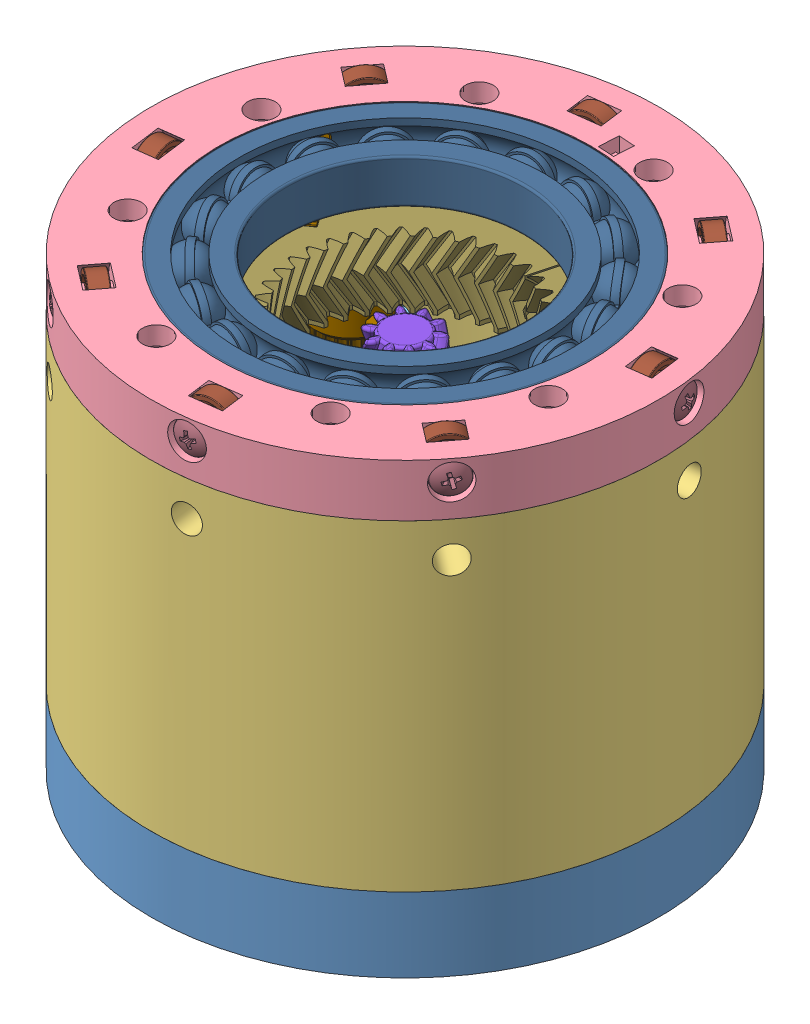
SolidWorks assembly A1 - Final Assembly, configuration Default. Lengths in mm.
Overall size (210.32 133.5 210.32).
45 component instances, 13 part files, 38 mates.
Components (placement in the parent):
- A1D1 - Bottom-1: A1D1 - Bottom [Default] at origin size (150 22 150)
- Turnigy Aerodrive SK3 4250-1: Turnigy Aerodrive SK3 4250 [Default] at (0 73.3 0) x (-0.707107 0 -0.707107) z (-0.707107 0 0.707107) size (52.1 79.08 41.8)
- A1D2 - Middle-1: A1D2 - Middle [Default] at (0 22 0) x (0.991445 0 -0.130526) z (0.130526 0 0.991445) size (150 96 150)
- A1D3 - Top-1: A1D3 - Top [Default] at (0 117 0) x (0.793353 0 0.608761) z (-0.608761 0 0.793353) size (150 15.5 150)
- A1D4 - Encoder bracket-1: A1D4 - Encoder bracket [Default] at (0 30 0) x (0.991445 0 -0.130526) z (0.130526 0 0.991445) size (52.04 50 76.58)
- Encoder600PR-1: Encoder600PR [Default] at (-40.4994 32.32 -24.4547) x (0.84353 0 0.537082) z (-0.537082 0 0.84353) size (38 53 38)
- A1P1_S1 - BLDC Axis Bottom (50T HTD3m)-1: A1P1_S1 - BLDC Axis Bottom (50T HTD3m) [Default] at (-3.3955 88.2939 1.3517) x (0.767493 0 -0.641057) z (0 -1 0) size (46.98 46.92 14.7)
- A1P1_S2 - BLDC Axis Top (Sun in A1R1)-1: A1P1_S2 - BLDC Axis Top (Sun in A1R1) [Default] at (-3.3955 88.2939 1.3517) x (0.767493 0 -0.641057) z (0 -1 0) size (38.1 38.1 28.24)
- A1P2 - Encoder Axis (20T HTD3m)-1: A1P2 - Encoder Axis (20T HTD3m) [Default] at (-40.4994 73.3 -24.4547) x (0.825705 0 -0.564102) z (0 1 0) size (21.34 40.98 60.33)
- radial ball bearing_68_am-3: radial ball bearing_68_am [AFBMA 20.1 - 00-70 - 18,DE,AC,18_68] at (0 126 0) x (0 1 0) z (0 0 1) size (13.2 110 110)
- radial ball bearing_68_iso-1: radial ball bearing_68_iso [ISO 15 RBB - 105 - 8,SI,NC,8_68] at (8.4842 126.5 64.4439) x (0.130526 0 0.991445) z (-0.991445 0 0.130526) size (5 14 14)
- radial ball bearing_68_iso-2: radial ball bearing_68_iso [ISO 15 RBB - 105 - 8,SI,NC,8_68] at (51.568 126.5 39.5695) x (0.793353 0 0.608761) z (-0.608761 0 0.793353) size (5 14 14)
- radial ball bearing_68_iso-3: radial ball bearing_68_iso [ISO 15 RBB - 105 - 8,SI,NC,8_68] at (64.4439 126.5 -8.4842) x (0.991445 0 -0.130526) z (0.130526 0 0.991445) size (5 14 14)
- radial ball bearing_68_iso-4: radial ball bearing_68_iso [ISO 15 RBB - 105 - 8,SI,NC,8_68] at (39.5695 126.5 -51.568) x (0.608761 0 -0.793353) z (0.793353 0 0.608761) size (5 14 14)
- radial ball bearing_68_iso-5: radial ball bearing_68_iso [ISO 15 RBB - 105 - 8,SI,NC,8_68] at (-8.4842 126.5 -64.4439) x (-0.130526 0 -0.991445) z (0.991445 0 -0.130526) size (5 14 14)
- radial ball bearing_68_iso-6: radial ball bearing_68_iso [ISO 15 RBB - 105 - 8,SI,NC,8_68] at (-51.568 126.5 -39.5695) x (-0.793353 0 -0.608761) z (0.608761 0 -0.793353) size (5 14 14)
- radial ball bearing_68_iso-7: radial ball bearing_68_iso [ISO 15 RBB - 105 - 8,SI,NC,8_68] at (-64.4439 126.5 8.4842) x (-0.991445 0 0.130526) z (-0.130526 0 -0.991445) size (5 14 14)
- radial ball bearing_68_iso-8: radial ball bearing_68_iso [ISO 15 RBB - 105 - 8,SI,NC,8_68] at (-39.5695 126.5 51.568) x (-0.608761 0 0.793353) z (-0.793353 0 -0.608761) size (5 14 14)
- A1R1 - Fixed ring (38T)-1: A1R1 - Fixed ring (38T) [Default] at (-96.4762 151.2552 -44.9758) x (0.965926 0 0.258819) z (0 1 0) size (84.14 84.14 19.84)
- pan head cross recess screw_iso-3: pan head cross recess screw_iso [ISO 7045 - M5 x 16 - Z - 16N] at (9.7764 126.5 74.2592) x (-0.130526 0 -0.991445) z (0.264332 -0.963804 -0.0348) size (19.63 9.5 9.5)
- pan head cross recess screw_iso-5: pan head cross recess screw_iso [ISO 7045 - M4 x 16 - Z - 16N] at (6.8787 106.5867 52.2491) x (-0.130526 0 -0.991445) z (-0.096727 -0.995229 0.012734) size (19.02 8 8)
- pan head cross recess screw_iso-6: pan head cross recess screw_iso [ISO 7045 - M4 x 16 - Z - 16N] at (30 128.5 51.9615) x (0 -1 0) z (0.614442 0 0.788962) size (19.02 8 8)
- pan head cross recess screw_iso-7: pan head cross recess screw_iso [ISO 7045 - M4 x 16 - Z - 16N] at (41.8097 106.5867 32.0817) x (-0.793353 0 -0.608761) z (-0.059392 -0.995229 0.077401) size (19.02 8 8)
- pan head cross recess screw_iso-8: pan head cross recess screw_iso [ISO 7045 - M4 x 16 - Z - 16N] at (52.2491 106.5867 -6.8787) x (-0.991445 0 0.130526) z (0.012734 -0.995229 0.096727) size (19.02 8 8)
- pan head cross recess screw_iso-9: pan head cross recess screw_iso [ISO 7045 - M4 x 16 - Z - 16N] at (32.0817 106.5867 -41.8097) x (-0.608761 0 0.793353) z (0.077401 -0.995229 0.059392) size (19.02 8 8)
- pan head cross recess screw_iso-10: pan head cross recess screw_iso [ISO 7045 - M4 x 16 - Z - 16N] at (-6.8787 106.5867 -52.2491) x (0.130526 0 0.991445) z (0.096727 -0.995229 -0.012734) size (19.02 8 8)
- pan head cross recess screw_iso-11: pan head cross recess screw_iso [ISO 7045 - M4 x 16 - Z - 16N] at (-41.8097 106.5867 -32.0817) x (0.793353 0 0.608761) z (0.059392 -0.995229 -0.077401) size (19.02 8 8)
- pan head cross recess screw_iso-12: pan head cross recess screw_iso [ISO 7045 - M4 x 16 - Z - 16N] at (-52.2491 106.5867 6.8787) x (0.991445 0 -0.130526) z (-0.012734 -0.995229 -0.096727) size (19.02 8 8)
- pan head cross recess screw_iso-13: pan head cross recess screw_iso [ISO 7045 - M4 x 16 - Z - 16N] at (-32.0817 106.5867 41.8097) x (0.608761 0 -0.793353) z (-0.077401 -0.995229 -0.059392) size (19.02 8 8)
- pan head cross recess screw_iso-14: pan head cross recess screw_iso [ISO 7045 - M4 x 16 - Z - 16N] at (57.9555 128.5 15.5291) x (0 -1 0) z (0.992357 0 0.123404) size (19.02 8 8)
- pan head cross recess screw_iso-15: pan head cross recess screw_iso [ISO 7045 - M4 x 16 - Z - 16N] at (51.9615 128.5 -30) x (0 -1 0) z (0.788962 0 -0.614442) size (19.02 8 8)
- pan head cross recess screw_iso-16: pan head cross recess screw_iso [ISO 7045 - M4 x 16 - Z - 16N] at (15.5291 128.5 -57.9555) x (0 -1 0) z (0.123404 0 -0.992357) size (19.02 8 8)
- pan head cross recess screw_iso-17: pan head cross recess screw_iso [ISO 7045 - M4 x 16 - Z - 16N] at (-30 128.5 -51.9615) x (0 -1 0) z (-0.614442 0 -0.788962) size (19.02 8 8)
- pan head cross recess screw_iso-18: pan head cross recess screw_iso [ISO 7045 - M4 x 16 - Z - 16N] at (-57.9555 128.5 -15.5291) x (0 -1 0) z (-0.992357 0 -0.123404) size (19.02 8 8)
- pan head cross recess screw_iso-19: pan head cross recess screw_iso [ISO 7045 - M4 x 16 - Z - 16N] at (-51.9615 128.5 30) x (0 -1 0) z (-0.788962 0 0.614442) size (19.02 8 8)
- pan head cross recess screw_iso-20: pan head cross recess screw_iso [ISO 7045 - M4 x 16 - Z - 16N] at (-15.5291 128.5 57.9555) x (0 -1 0) z (-0.123404 0 0.992357) size (19.02 8 8)
- pan head cross recess screw_iso-21: pan head cross recess screw_iso [ISO 7045 - M5 x 16 - Z - 16N] at (59.4222 126.5 45.5962) x (-0.793353 0 -0.608761) z (0.162304 -0.963804 -0.211518) size (19.63 9.5 9.5)
- pan head cross recess screw_iso-22: pan head cross recess screw_iso [ISO 7045 - M5 x 16 - Z - 16N] at (74.2592 126.5 -9.7764) x (-0.991445 0 0.130526) z (-0.0348 -0.963804 -0.264332) size (19.63 9.5 9.5)
- pan head cross recess screw_iso-23: pan head cross recess screw_iso [ISO 7045 - M5 x 16 - Z - 16N] at (45.5962 126.5 -59.4222) x (-0.608761 0 0.793353) z (-0.211518 -0.963804 -0.162304) size (19.63 9.5 9.5)
- pan head cross recess screw_iso-24: pan head cross recess screw_iso [ISO 7045 - M5 x 16 - Z - 16N] at (-9.7764 126.5 -74.2592) x (0.130526 0 0.991445) z (-0.264332 -0.963804 0.0348) size (19.63 9.5 9.5)
- pan head cross recess screw_iso-25: pan head cross recess screw_iso [ISO 7045 - M5 x 16 - Z - 16N] at (-59.4222 126.5 -45.5962) x (0.793353 0 0.608761) z (-0.162304 -0.963804 0.211518) size (19.63 9.5 9.5)
- pan head cross recess screw_iso-26: pan head cross recess screw_iso [ISO 7045 - M5 x 16 - Z - 16N] at (-74.2592 126.5 9.7764) x (0.991445 0 -0.130526) z (0.0348 -0.963804 0.264332) size (19.63 9.5 9.5)
- pan head cross recess screw_iso-27: pan head cross recess screw_iso [ISO 7045 - M5 x 16 - Z - 16N] at (-45.5962 126.5 59.4222) x (0.608761 0 -0.793353) z (0.211518 -0.963804 0.162304) size (19.63 9.5 9.5)
- pan head cross recess screw_iso-29: pan head cross recess screw_iso [ISO 7045 - M5 x 16 - Z - 16N] at (-75.73 69.5 20.0563) x (0.991445 0 -0.130526) z (-0.041237 0.948782 -0.313228) size (19.63 9.5 9.5)
- pan head cross recess screw_iso-30: pan head cross recess screw_iso [ISO 7045 - M5 x 16 - Z - 16N] at (-78.3405 69.5 0.2274) x (0.991445 0 -0.130526) z (0.119155 0.408217 0.905075) size (19.63 9.5 9.5)
Mates (geometry in assembly coordinates):
- Concentric1: concentric anti-aligned: cylinder of A1D1 - Bottom-1 through (-12.5 16 0) axis (0 1 0) radius 1.6; cylinder of Turnigy Aerodrive SK3 4250-1 through (-12.5 24 0) axis (0 -1 0) radius 1.5
- Concentric2: concentric anti-aligned: cylinder of A1D1 - Bottom-1 through (12.5 16 0) axis (0 1 0) radius 1.6; cylinder of Turnigy Aerodrive SK3 4250-1 through (12.5 24 0) axis (0 -1 0) radius 1.5
- Coincident1: coincident anti-aligned: plane of A1D1 - Bottom-1 through (0 22 0) normal (0 1 0); plane of Turnigy Aerodrive SK3 4250-1 through (0 22 0) normal (0 -1 0)
- Concentric3: concentric aligned: cylinder of A1D1 - Bottom-1 through (30 -31.885 51.9615) axis (0 1 0) radius 2.05; cylinder of A1D2 - Middle-1 through (30 21.999 51.9615) axis (0 1 0) radius 2.05
- Concentric4: concentric aligned: cylinder of A1D1 - Bottom-1 through (60 -23.7417 0) axis (0 1 0) radius 2.05; cylinder of A1D2 - Middle-1 through (60 21.999 0) axis (0 1 0) radius 2.05
- Coincident2: coincident anti-aligned: plane of A1D1 - Bottom-1 through (0 22 0) normal (0 1 0); plane of A1D2 - Middle-1 through (-9.7895 22 -74.3584) normal (0 -1 0)
- Concentric5: concentric aligned: cylinder of A1D2 - Middle-1 through (0 22 0) axis (0 -1 0) radius 75; cylinder of A1D3 - Top-1 through (0 132.5 0) axis (0 -1 0) radius 75
- Coincident3: coincident anti-aligned: plane of A1D2 - Middle-1 through (-5.717 117 -43.4253) normal (0 1 0); plane of A1D3 - Top-1 through (0 117 0) normal (0 -1 0)
- Concentric6: concentric aligned: cylinder of A1D2 - Middle-1 through (30 21.999 51.9615) axis (0 1 0) radius 2.05; cylinder of A1D3 - Top-1 through (30 117 51.9615) axis (0 1 0) radius 2.05
- Concentric7: concentric anti-aligned: cylinder of A1D2 - Middle-1 through (-73.0541 69.5 19.704) axis (0.991445 0 -0.130526) radius 2.55; cylinder of A1D4 - Encoder bracket-1 through (16.6736 69.5 7.8912) axis (-0.991445 0 0.130526) radius 2.55
- Concentric8: concentric aligned: cylinder of A1D2 - Middle-1 through (0 22 0) axis (0 -1 0) radius 70; cylinder of A1D4 - Encoder bracket-1 through (0 80 0) axis (0 -1 0) radius 70
- Concentric9: concentric anti-aligned: cylinder of A1D4 - Encoder bracket-1 through (-40.4994 21.499 -24.4547) axis (0 1 0) radius 11; cylinder of Encoder600PR-1 through (-40.4994 67.32 -24.4547) axis (0 -1 0) radius 19
- Coincident4: coincident anti-aligned: plane of A1D4 - Encoder bracket-1 through (0 67.32 0) normal (0 -1 0); plane of Encoder600PR-1 through (-40.4994 67.32 -24.4547) normal (0 1 0)
- Concentric10: concentric aligned: cylinder of A1D4 - Encoder bracket-1 through (-34.0317 21.499 -12.0382) axis (0 1 0) radius 1.5; cylinder of Encoder600PR-1 through (-34.0317 51.32 -12.0382) axis (0 1 0) radius 1.5
- Concentric11: concentric anti-aligned: cylinder of A1P1_S1 - BLDC Axis Bottom (50T HTD3m)-1 through (0 70.1 0) axis (0 1 0) radius 11; cylinder of A1P1_S2 - BLDC Axis Top (Sun in A1R1)-1 through (0 92.97 0) axis (0 -1 0) radius 9.165
- Concentric12: concentric anti-aligned: cylinder of A1P1_S1 - BLDC Axis Bottom (50T HTD3m)-1 through (10.2569 70.1 12.2799) axis (0 1 0) radius 1.55; cylinder of A1P1_S2 - BLDC Axis Top (Sun in A1R1)-1 through (10.2569 87.8 12.2799) axis (0 -1 0) radius 1.55
- Coincident6: coincident anti-aligned: plane of A1P1_S1 - BLDC Axis Bottom (50T HTD3m)-1 through (9.5092 84.8 19.9621) normal (0 1 0); plane of A1P1_S2 - BLDC Axis Top (Sun in A1R1)-1 through (9.5092 84.8 19.9621) normal (0 -1 0)
- Concentric13: concentric anti-aligned: cylinder of Turnigy Aerodrive SK3 4250-1 through (0 76.8 0) axis (0 1 0) radius 5.5; cylinder of A1P1_S1 - BLDC Axis Bottom (50T HTD3m)-1 through (0 77.1 0) axis (0 -1 0) radius 5.7
- Parallel2: parallel aligned: cylinder of Turnigy Aerodrive SK3 4250-1 through (7.4859 68.3 2.0058) axis (0 1 0) radius 1.25; cylinder of A1P1_S1 - BLDC Axis Bottom (50T HTD3m)-1 through (5.5062 70.1 -15.0227) axis (0 1 0) radius 1.55
- Coincident7: coincident anti-aligned: plane of Turnigy Aerodrive SK3 4250-1 through (0 73.3 0) normal (0 1 0); plane of A1P1_S1 - BLDC Axis Bottom (50T HTD3m)-1 through (-33.8971 73.3 1.3219) normal (0 -1 0)
- Concentric16: concentric anti-aligned: cylinder of Encoder600PR-1 through (-40.4994 85.32 -24.4547) axis (0 -1 0) radius 3; cylinder of A1P2 - Encoder Axis (20T HTD3m)-1 through (-40.4994 70.3 -24.4547) axis (0 1 0) radius 2.6
- Coincident8: coincident aligned: plane of A1P1_S1 - BLDC Axis Bottom (50T HTD3m)-1 through (-33.8971 73.3 1.3219) normal (0 -1 0); plane of A1P2 - Encoder Axis (20T HTD3m)-1 through (-40.4994 73.3 -24.4547) normal (0 -1 0)
- Concentric18: concentric anti-aligned: cylinder of A1D3 - Top-1 through (0 132.5 0) axis (0 -1 0) radius 54.925; cylinder of radial ball bearing_68_am-3 through (0 105.3625 0) axis (0 1 0) radius 55
- Coincident9: coincident anti-aligned: plane of A1D3 - Top-1 through (0 119.5 0) normal (0 1 0); plane of radial ball bearing_68_am-3 through (-49 119.5 0) normal (0 -1 0)
- Concentric19: concentric anti-aligned: cylinder of A1D3 - Top-1 through (9.0716 126.5 68.9054) axis (-0.130526 0 -0.991445) radius 2.55; cylinder of radial ball bearing_68_iso-1 through (5.7905 126.5 43.983) axis (0.130526 0 0.991445) radius 2.5
- Coincident10: coincident anti-aligned: plane of A1D3 - Top-1 through (8.1579 126.5 61.9653) normal (0.130526 0 0.991445); plane of radial ball bearing_68_iso-1 through (8.1579 130.35 61.9653) normal (-0.130526 0 -0.991445)
- Concentric20: concentric anti-aligned: cylinder of radial ball bearing_68_am-3 through (0 105.3625 0) axis (0 1 0) radius 35; circle of A1R1 - Fixed ring (38T)-1
- Concentric22: concentric aligned: cylinder of A1D2 - Middle-1 through (84.149 106.5867 64.5698) axis (-0.793353 0 -0.608761) radius 2; cylinder of A1R1 - Fixed ring (38T)-1 through (-26.5773 106.5867 -20.3935) axis (-0.793353 0 -0.608761) radius 2.05
- Concentric24: concentric aligned: cylinder of A1D3 - Top-1 through (9.2935 126.5 70.5909) axis (0.130526 0 0.991445) radius 5.1; cylinder of pan head cross recess screw_iso-3 through (13.0918 126.5 99.4419) axis (0.130526 0 0.991445) radius 4.75
- Coincident12: coincident anti-aligned: plane of A1D3 - Top-1 through (9.2935 126.5 70.5909) normal (0.130526 0 0.991445); plane of pan head cross recess screw_iso-3 through (11.6824 127.1665 70.2764) normal (-0.130526 0 -0.991445)
- Concentric25: concentric aligned: cylinder of A1D2 - Middle-1 through (6.4741 106.5867 49.1757) axis (0.130526 0 0.991445) radius 4.1; cylinder of pan head cross recess screw_iso-5 through (10.1941 106.5867 77.4318) axis (0.130526 0 0.991445) radius 2
- Coincident13: coincident anti-aligned: plane of A1D2 - Middle-1 through (6.4741 106.5867 49.1757) normal (0.130526 0 0.991445); plane of pan head cross recess screw_iso-5 through (8.4475 106.3915 48.9159) normal (-0.130526 0 -0.991445)
- Concentric26: concentric aligned: cylinder of A1D3 - Top-1 through (30 117 51.9615) axis (0 1 0) radius 2.05; cylinder of pan head cross recess screw_iso-6 through (30 153.9 51.9615) axis (0 1 0) radius 2
- Coincident14: coincident anti-aligned: plane of A1D3 - Top-1 through (30 125.4 51.9615) normal (0 1 0); plane of pan head cross recess screw_iso-6 through (31.5779 125.4 50.7326) normal (0 -1 0)
- Concentric28: concentric anti-aligned: cylinder of A1D2 - Middle-1 through (-73.0541 69.5 19.704) axis (0.991445 0 -0.130526) radius 2.55; cylinder of pan head cross recess screw_iso-29 through (-100.9127 69.5 23.3717) axis (-0.991445 0 0.130526) radius 2.5
- Tangent1: tangent anti-aligned: cylinder of A1D2 - Middle-1 through (0 22 0) axis (0 -1 0) radius 74; plane of pan head cross recess screw_iso-29 through (-72.3713 68.7102 17.2217) normal (0.991445 0 -0.130526)
- Concentric29: concentric anti-aligned: cylinder of A1D2 - Middle-1 through (-75.6646 69.5 -0.1249) axis (0.991445 0 -0.130526) radius 2.55; cylinder of pan head cross recess screw_iso-30 through (-103.5232 69.5 3.5428) axis (-0.991445 0 0.130526) radius 2.5
- Tangent2: tangent anti-aligned: cylinder of A1D2 - Middle-1 through (0 22 0) axis (0 -1 0) radius 74; plane of pan head cross recess screw_iso-30 through (-74.8054 71.7822 -1.2673) normal (0.991445 0 -0.130526)
